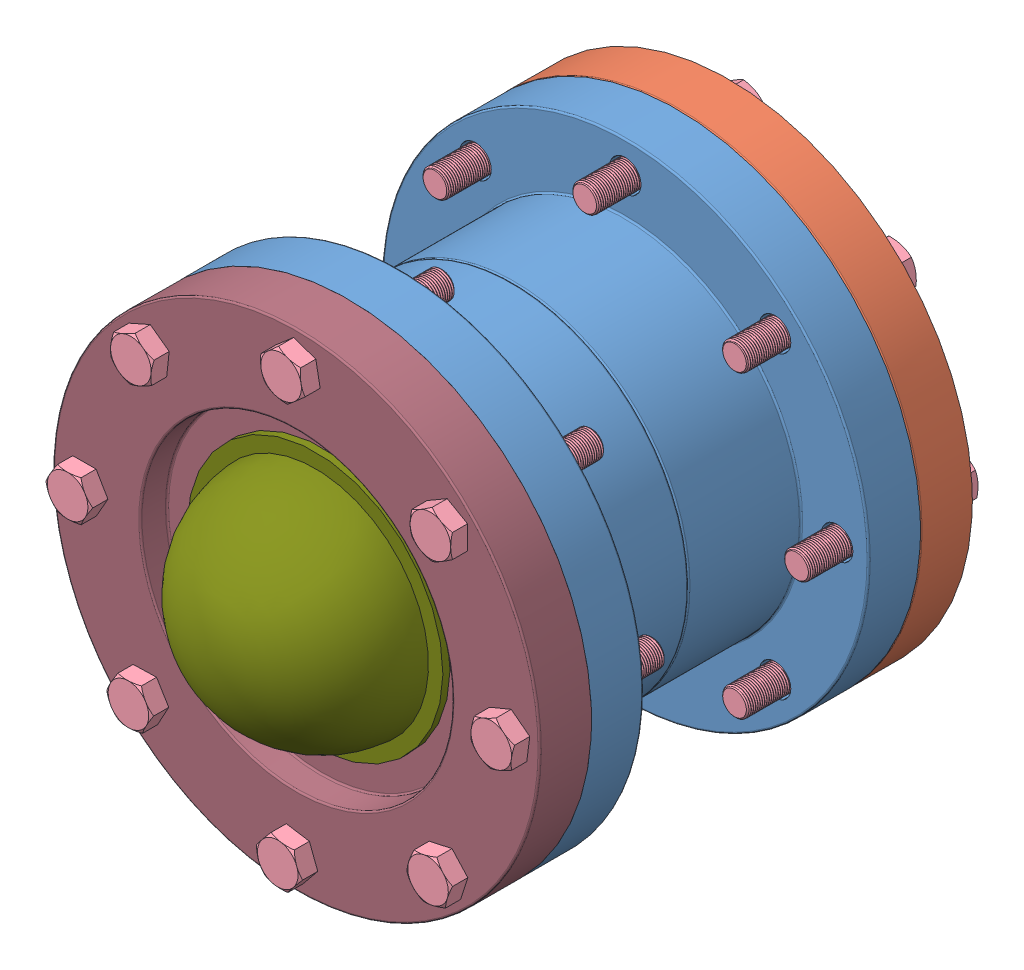
SolidWorks assembly Photogrametry_V5-PVC, configuration Default. Lengths in mm.
Overall size (484.92 484.92 378.41).
39 component instances, 16 part files, 25 mates.
Components (placement in the parent):
- externalHousing-Assembly-1: externalHousing-Assembly [Default] at (41.8532 87.3209 72.2129) size (484.92 484.92 280.15)
  - 8in PVC Flange-1: 8in PVC Flange [4881K224] at (120.5656 188.2131 202.8846) size (342.9 342.9 115.89)
  - 8in PVC Flange Closed-1: 8in PVC Flange Closed [4881K973] at (120.5656 188.2131 166.3721) size (342.9 342.9 36.51)
  - 8in PVC Pipe-1: 8in PVC Pipe [48855K43] at (120.5656 188.2131 318.8302) x (0.914978 0.403503 0) z (0 0 1) size (219.07 219.07 203.2)
  - 8in PVC Flange-2: 8in PVC Flange [4881K224] at (120.5656 188.2131 434.6169) x (-0.71277 -0.701398 0) z (0 0 -1) size (342.9 342.9 115.89)
  - BOLT 3-4in x 4in-1: BOLT 3-4in x 4in [92198A390] at (120.5656 337.4381 211.219) x (0 0 1) z (-0.999812 -0.019405 0) size (114.21 33 28.57)
  - BOLT 3-4in x 4in-2: BOLT 3-4in x 4in [92198A390] at (120.5656 38.9881 211.219) x (0 0 1) z (-0.865453 -0.50099 0) size (114.21 33 28.57)
  - BOLT 3-4in x 4in-3: BOLT 3-4in x 4in [92198A390] at (269.7906 188.2131 211.219) x (0 0 1) z (-0.997964 -0.063786 0) size (114.21 33 28.57)
  - BOLT 3-4in x 4in-4: BOLT 3-4in x 4in [92198A390] at (226.0836 82.6951 211.219) x (0 0 1) z (-0.850633 -0.525759 0) size (114.21 33 28.57)
  - BOLT 3-4in x 4in-5: BOLT 3-4in x 4in [92198A390] at (-28.6594 188.2131 211.219) x (0 0 1) z (-0.888414 -0.459043 0) size (114.21 33 28.57)
  - BOLT 3-4in x 4in-6: BOLT 3-4in x 4in [92198A390] at (15.0476 293.7311 211.219) x (0 0 1) z (-0.838585 0.544771 0) size (114.21 33 28.57)
  - BOLT 3-4in x 4in-7: BOLT 3-4in x 4in [92198A390] at (15.0476 82.6951 211.219) x (0 0 1) z (-0.991201 -0.132366 0) size (114.21 33 28.57)
  - BOLT 3-4in x 4in-8: BOLT 3-4in x 4in [92198A390] at (226.0836 293.7311 211.219) x (0 0 1) z (-0.666953 0.7451 0) size (114.21 33 28.57)
- piston-Assembly-1: piston-Assembly [Default] at (263.1271 385.721 271.7537) x (-0.99718 0.075046 0) z (0 0 1) size (196.82 196.82 115.45)
  - piston-BackRing-1: piston-BackRing [Default] at (92.1552 117.4341 124.8546) size (190 190 16)
  - piston-CameraPlate-1: piston-CameraPlate [Default] at (92.1552 53.6841 162.8546) size (140 30 60)
  - piston-FrontRing-1: piston-FrontRing [Default] at (92.1552 117.4341 200.8546) size (190 190 16)
  - piston-SpacerTube-1: piston-SpacerTube [Default] at (92.1552 187.4341 132.8546) x (-0.829647 0.558289 0) z (0 0 1) size (18 18 60)
  - BOLT M8x110mm-1: BOLT M8x110mm [91287A317] at (42.1552 68.6841 156.5046) size (13 15.01 115.45)
  - BOLT M8x110mm-2: BOLT M8x110mm [91287A317] at (142.1552 68.6841 156.5046) x (0.995976 0.089615 0) z (0 0 1) size (13 15.01 115.45)
  - BOLT M8x110mm-3: BOLT M8x110mm [91287A317] at (92.1552 187.4341 156.5046) x (0.993023 -0.117919 0) z (0 0 1) size (13 15.01 115.45)
  - piston-7inO-RING-1: piston-7inO-RING [9452K426] at (91.7077 116.5016 200.4895) x (0.999544 -0.030202 0) z (0 0 1) size (191.13 191.13 6.99)
  - piston-7inO-RING-2: piston-7inO-RING [9452K426] at (91.7417 116.9322 125.1185) size (191.13 191.13 6.99)
- ROD M8 150mm-1: ROD M8 150mm [98861A593] at (191.0068 322.2703 396.8412) x (0 0 -1) z (1 0 0) size (281.88 8 9.24)
- SPRING-1: SPRING [94125K22] at (191.2399 321.4655 334.2689) x (1 0 0) z (0 0.999848 0.017452) size (11.51 82 11.48)
- 8in PVC Flange Closed - Dome Mount Cut-2: 8in PVC Flange Closed - Dome Mount Cut [4881K973] at (162.4188 275.534 506.8298) x (0.999968 -0.008041 0) z (0 0 1) size (342.9 342.9 36.51)
- BOLT 3-4in x 4in-1: BOLT 3-4in x 4in [92198A390] at (163.6187 424.7542 498.4954) x (0 0 -1) z (0.32993 0.944005 0) size (114.21 33 28.57)
- BOLT 3-4in x 4in-2: BOLT 3-4in x 4in [92198A390] at (57.7526 381.897 498.4954) x (0 0 -1) z (0.589733 0.807598 0) size (114.21 33 28.57)
- BOLT 3-4in x 4in-3: BOLT 3-4in x 4in [92198A390] at (13.1986 276.7338 498.4954) x (0 0 -1) z (0.863135 0.504973 0) size (114.21 33 28.57)
- BOLT 3-4in x 4in-4: BOLT 3-4in x 4in [92198A390] at (56.0557 170.8678 498.4954) x (0 0 -1) z (0.852954 0.521986 0) size (114.21 33 28.57)
- BOLT 3-4in x 4in-5: BOLT 3-4in x 4in [92198A390] at (268.7818 380.2001 498.4954) x (0 0 -1) z (0.494985 0.868902 0) size (114.21 33 28.57)
- BOLT 3-4in x 4in-6: BOLT 3-4in x 4in [92198A390] at (311.639 274.3341 498.4954) x (0 0 -1) z (0.607098 0.794627 0) size (114.21 33 28.57)
- BOLT 3-4in x 4in-7: BOLT 3-4in x 4in [92198A390] at (161.2189 126.3138 498.4954) x (0 0 -1) z (0.933987 0.357308 0) size (114.21 33 28.57)
- BOLT 3-4in x 4in-8: BOLT 3-4in x 4in [92198A390] at (267.0849 169.1709 498.4954) x (0 0 -1) z (0.738489 0.674266 0) size (114.21 33 28.57)
- A7 III + FE 28-70 v4-1: A7 III + FE 28-70 v4 [Default] at (177.6736 311.0552 442.428) x (-0.998469 0.054614 -0.008727) z (-0.054538 -0.998474 -0.008726) size (139.07 134.7 103.31)
  - A7 III + FE 28-70 v4.step-1: A7 III + FE 28-70 v4.step [Default] at origin size (139.07 134.7 103.31)
    - Sony A7 III.step-1: Sony A7 III.step [Default] at origin size (139.07 74.69 103.31)
    - Sony FE 28-70 mm f_3.5-5.6 OSS.step-1: Sony FE 28-70 mm f_3.5-5.6 OSS.step [Default] at (13.5 -93.5 40) size (72.5 83 72.5)
- Custom Dome-1: Custom Dome [Default] at (162.4188 275.534 525.086) x (0.91761 0.397483 0) z (0.397483 -0.91761 0) size (180 80 180)
Mates (geometry in assembly coordinates):
- Lock1: lock: unknown of ROD M8 150mm-1; unknown of SPRING-1
- Concentric1: concentric anti-aligned: circle of piston-Assembly-1/piston-FrontRing-1; circle of ROD M8 150mm-1
- Concentric3: concentric aligned: circle of externalHousing-Assembly-1/8in PVC Flange-2; circle of piston-Assembly-1/piston-BackRing-1
- Coincident2: coincident anti-aligned: plane of externalHousing-Assembly-1/8in PVC Flange Closed-1 through (162.4188 384.881 256.8412) normal (0 0 1); plane of ROD M8 150mm-1 through (191.0068 322.2703 256.8412) normal (0 0 -1)
- Coincident4: coincident anti-aligned: circle of 8in PVC Flange Closed - Dome Mount Cut-2; circle of externalHousing-Assembly-1/8in PVC Flange-2
- Coincident6: coincident anti-aligned: circle of externalHousing-Assembly-1/8in PVC Flange-2; circle of 8in PVC Flange Closed - Dome Mount Cut-2
- Concentric5: concentric anti-aligned: circle of 8in PVC Flange Closed - Dome Mount Cut-2; circle of BOLT 3-4in x 4in-5
- Coincident7: coincident anti-aligned: plane of 8in PVC Flange Closed - Dome Mount Cut-2 through (162.4188 275.534 543.3423) normal (0 0 1); plane of BOLT 3-4in x 4in-5 through (268.6864 396.6976 543.3423) normal (0 0 -1)
- Concentric6: concentric anti-aligned: circle of 8in PVC Flange Closed - Dome Mount Cut-2; circle of BOLT 3-4in x 4in-1
- Coincident8: coincident anti-aligned: plane of 8in PVC Flange Closed - Dome Mount Cut-2 through (162.4188 275.534 543.3423) normal (0 0 1); plane of BOLT 3-4in x 4in-1 through (160.5455 440.9632 543.3423) normal (0 0 -1)
- Concentric7: concentric anti-aligned: circle of 8in PVC Flange Closed - Dome Mount Cut-2; circle of BOLT 3-4in x 4in-2
- Coincident9: coincident anti-aligned: plane of 8in PVC Flange Closed - Dome Mount Cut-2 through (162.4188 275.534 543.3423) normal (0 0 1); plane of BOLT 3-4in x 4in-2 through (59.5166 398.3002 543.3423) normal (0 0 -1)
- Concentric8: concentric anti-aligned: circle of 8in PVC Flange Closed - Dome Mount Cut-2; circle of BOLT 3-4in x 4in-3
- Coincident10: coincident anti-aligned: plane of 8in PVC Flange Closed - Dome Mount Cut-2 through (162.4188 275.534 543.3423) normal (0 0 1); plane of BOLT 3-4in x 4in-3 through (21.3652 291.0686 543.3423) normal (0 0 -1)
- Concentric9: concentric anti-aligned: circle of 8in PVC Flange Closed - Dome Mount Cut-2; circle of BOLT 3-4in x 4in-6
- Coincident11: coincident anti-aligned: plane of 8in PVC Flange Closed - Dome Mount Cut-2 through (162.4188 275.534 543.3423) normal (0 0 1); plane of BOLT 3-4in x 4in-6 through (313.7581 290.6952 543.3423) normal (0 0 -1)
- Concentric10: concentric anti-aligned: circle of 8in PVC Flange Closed - Dome Mount Cut-2; circle of BOLT 3-4in x 4in-4
- Coincident12: coincident anti-aligned: plane of 8in PVC Flange Closed - Dome Mount Cut-2 through (162.4188 275.534 543.3423) normal (0 0 1); plane of BOLT 3-4in x 4in-4 through (63.9365 185.3616 543.3423) normal (0 0 -1)
- Concentric11: concentric anti-aligned: circle of 8in PVC Flange Closed - Dome Mount Cut-2; circle of BOLT 3-4in x 4in-7
- Coincident13: coincident anti-aligned: plane of 8in PVC Flange Closed - Dome Mount Cut-2 through (162.4188 275.534 543.3423) normal (0 0 1); plane of BOLT 3-4in x 4in-7 through (171.6159 139.1232 543.3423) normal (0 0 -1)
- Concentric12: concentric anti-aligned: circle of 8in PVC Flange Closed - Dome Mount Cut-2; circle of BOLT 3-4in x 4in-8
- Coincident14: coincident anti-aligned: plane of 8in PVC Flange Closed - Dome Mount Cut-2 through (162.4188 275.534 543.3423) normal (0 0 1); plane of BOLT 3-4in x 4in-8 through (272.0741 184.8962 543.3423) normal (0 0 -1)
- Lock2: lock: unknown of piston-Assembly-1/piston-FrontRing-1; unknown of A7 III + FE 28-70 v4-1/A7 III + FE 28-70 v4.step-1/Sony A7 III.step-1
- Concentric13: concentric: circle of 8in PVC Flange Closed - Dome Mount Cut-2; circle of Custom Dome-1
- Coincident16: coincident anti-aligned: plane of 8in PVC Flange Closed - Dome Mount Cut-2 through (163.298 384.8774 525.086) normal (0 0 1); plane of Custom Dome-1 through (79.8339 239.7606 525.086) normal (0 0 -1)
